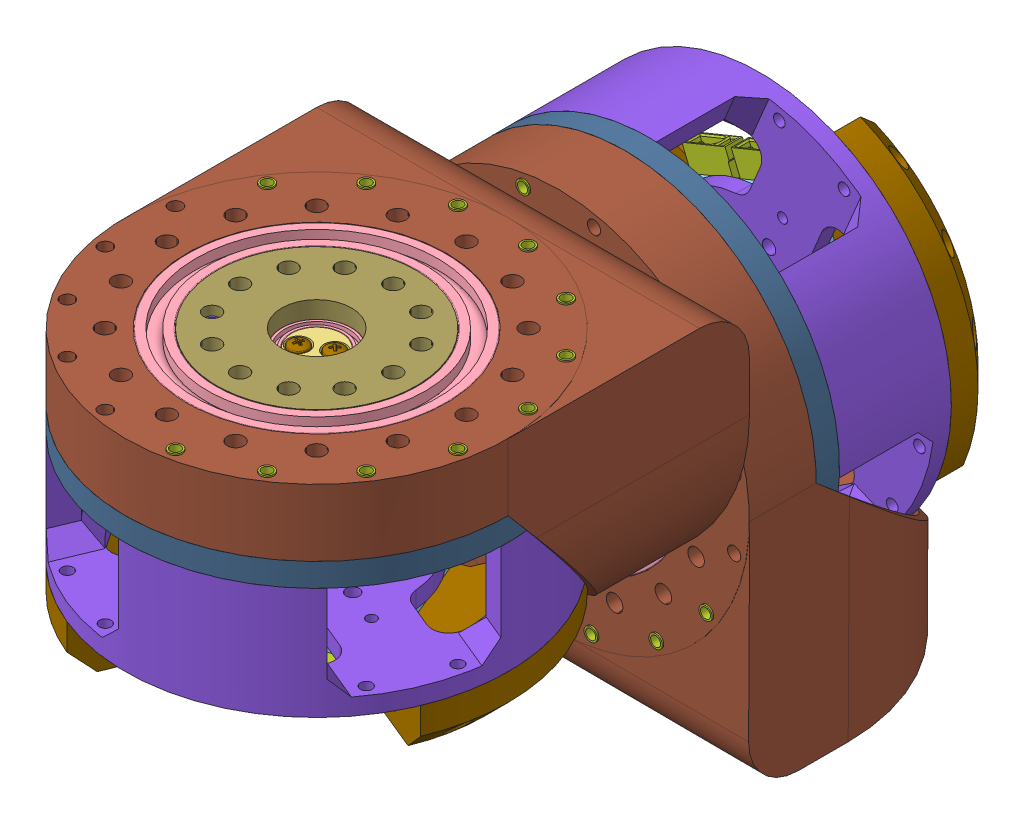
SolidWorks assembly hip, configuration Default. Lengths in mm.
Overall size (151.07 151.07 235.19).
696 component instances, 93 part files, 3 mates.
Components (placement in the parent):
- Cycloidal_v3-1: Cycloidal_v3 [Default] at (-2.6595 13.4678 32.6634) size (150.25 88 150.25)
  - motor-X83008S.stp-1: motor-X83008S.stp [Default] at (85.5027 89.8915 67.8666) x (-0.706334 0 0.707879) z (0 -1 0) size (114.7 114.7 37.62) (hidden)
    - base.stp-1: base.stp [Default] at (42.0794 12.0269 46.7342) size (91.6 91.6 15.61)
    - stator.stp-1: stator.stp [Default] at (42.0794 12.0269 33.1342) x (0.08493 -0.996387 0) z (0 0 1) size (83 83 8)
    - coil.stp-1: coil.stp [Default] at (39.5332 41.8984 37.1342) x (0.996387 0.08493 0) z (-0.08493 0.996387 0) size (4.4 10.2 10.5)
    - coil.stp-2: coil.stp [Default] at (34.3848 41.0025 37.1342) x (0.966502 0.256661 0) z (-0.256661 0.966502 0) size (4.4 10.2 10.5)
    - coil.stp-3: coil.stp [Default] at (29.4701 39.2261 37.1342) x (0.90725 0.420593 0) z (-0.420593 0.90725 0) size (4.4 10.2 10.5)
    - coil.stp-4: coil.stp [Default] at (24.9386 36.6233 37.1342) x (0.820431 0.571745 0) z (-0.571745 0.820431 0) size (4.4 10.2 10.5)
    - coil.stp-5: coil.stp [Default] at (20.9279 33.2732 37.1342) x (0.708685 0.705525 0) z (-0.705525 0.708685 0) size (4.4 10.2 10.5)
    - coil.stp-6: coil.stp [Default] at (17.5599 29.2775 37.1342) x (0.575405 0.817869 0) z (-0.817869 0.575405 0) size (4.4 10.2 10.5)
    - coil.stp-7: coil.stp [Default] at (14.9368 24.7576 37.1342) x (0.424642 0.905361 0) z (-0.905361 0.424642 0) size (4.4 10.2 10.5)
    - coil.stp-8: coil.stp [Default] at (13.1385 19.8509 37.1342) x (0.260976 0.965345 0) z (-0.965345 0.260976 0) size (4.4 10.2 10.5)
    - coil.stp-9: coil.stp [Default] at (12.2196 14.7066 37.1342) x (0.089381 0.995998 0) z (-0.995998 0.089381 0) size (4.4 10.2 10.5)
    - coil.stp-10: coil.stp [Default] at (12.2079 9.4807 37.1342) x (-0.08493 0.996387 0) z (-0.996387 -0.08493 0) size (4.4 10.2 10.5)
    - coil.stp-11: coil.stp [Default] at (13.1039 4.3323 37.1342) x (-0.256661 0.966502 0) z (-0.966502 -0.256661 0) size (4.4 10.2 10.5)
    - coil.stp-12: coil.stp [Default] at (14.8802 -0.5824 37.1342) x (-0.420593 0.90725 0) z (-0.90725 -0.420593 0) size (4.4 10.2 10.5)
    - coil.stp-13: coil.stp [Default] at (17.483 -5.1139 37.1342) x (-0.571745 0.820431 0) z (-0.820431 -0.571745 0) size (4.4 10.2 10.5)
    - coil.stp-14: coil.stp [Default] at (20.8332 -9.1246 37.1342) x (-0.705525 0.708685 0) z (-0.708685 -0.705525 0) size (4.4 10.2 10.5)
    - coil.stp-15: coil.stp [Default] at (24.8289 -12.4926 37.1342) x (-0.817869 0.575405 0) z (-0.575405 -0.817869 0) size (4.4 10.2 10.5)
    - coil.stp-16: coil.stp [Default] at (29.3487 -15.1157 37.1342) x (-0.905361 0.424642 0) z (-0.424642 -0.905361 0) size (4.4 10.2 10.5)
    - coil.stp-17: coil.stp [Default] at (34.2554 -16.914 37.1342) x (-0.965345 0.260976 0) z (-0.260976 -0.965345 0) size (4.4 10.2 10.5)
    - coil.stp-18: coil.stp [Default] at (39.3998 -17.8329 37.1342) x (-0.995998 0.089381 0) z (-0.089381 -0.995998 0) size (4.4 10.2 10.5)
    - coil.stp-19: coil.stp [Default] at (44.6256 -17.8446 37.1342) x (-0.996387 -0.08493 0) z (0.08493 -0.996387 0) size (4.4 10.2 10.5)
    - coil.stp-20: coil.stp [Default] at (49.7741 -16.9486 37.1342) x (-0.966502 -0.256661 0) z (0.256661 -0.966502 0) size (4.4 10.2 10.5)
    - coil.stp-21: coil.stp [Default] at (54.6887 -15.1723 37.1342) x (-0.90725 -0.420593 0) z (0.420593 -0.90725 0) size (4.4 10.2 10.5)
    - coil.stp-22: coil.stp [Default] at (59.2202 -12.5695 37.1342) x (-0.820431 -0.571745 0) z (0.571745 -0.820431 0) size (4.4 10.2 10.5)
    - coil.stp-23: coil.stp [Default] at (63.2309 -9.2193 37.1342) x (-0.708685 -0.705525 0) z (0.705525 -0.708685 0) size (4.4 10.2 10.5)
    - coil.stp-24: coil.stp [Default] at (66.599 -5.2236 37.1342) x (-0.575405 -0.817869 0) z (0.817869 -0.575405 0) size (4.4 10.2 10.5)
    - coil.stp-25: coil.stp [Default] at (69.222 -0.7038 37.1342) x (-0.424642 -0.905361 0) z (0.905361 -0.424642 0) size (4.4 10.2 10.5)
    - coil.stp-26: coil.stp [Default] at (71.0203 4.2029 37.1342) x (-0.260976 -0.965345 0) z (0.965345 -0.260976 0) size (4.4 10.2 10.5)
    - coil.stp-27: coil.stp [Default] at (71.9392 9.3473 37.1342) x (-0.089381 -0.995998 0) z (0.995998 -0.089381 0) size (4.4 10.2 10.5)
    - coil.stp-28: coil.stp [Default] at (71.9509 14.5731 37.1342) x (0.08493 -0.996387 0) z (0.996387 0.08493 0) size (4.4 10.2 10.5)
    - coil.stp-29: coil.stp [Default] at (71.055 19.7216 37.1342) x (0.256661 -0.966502 0) z (0.966502 0.256661 0) size (4.4 10.2 10.5)
    - coil.stp-30: coil.stp [Default] at (69.2786 24.6362 37.1342) x (0.420593 -0.90725 0) z (0.90725 0.420593 0) size (4.4 10.2 10.5)
    - coil.stp-31: coil.stp [Default] at (66.6758 29.1677 37.1342) x (0.571745 -0.820431 0) z (0.820431 0.571745 0) size (4.4 10.2 10.5)
    - coil.stp-32: coil.stp [Default] at (63.3257 33.1785 37.1342) x (0.705525 -0.708685 0) z (0.708685 0.705525 0) size (4.4 10.2 10.5)
    - coil.stp-33: coil.stp [Default] at (59.33 36.5465 37.1342) x (0.817869 -0.575405 0) z (0.575405 0.817869 0) size (4.4 10.2 10.5)
    - coil.stp-34: coil.stp [Default] at (54.8101 39.1695 37.1342) x (0.905361 -0.424642 0) z (0.424642 0.905361 0) size (4.4 10.2 10.5)
    - coil.stp-35: coil.stp [Default] at (49.9034 40.9678 37.1342) x (0.965345 -0.260976 0) z (0.260976 0.965345 0) size (4.4 10.2 10.5)
    - coil.stp-36: coil.stp [Default] at (44.759 41.8868 37.1342) x (0.995998 -0.089381 0) z (0.089381 0.995998 0) size (4.4 10.2 10.5)
    - rotor.stp-1: rotor.stp [Default] at (42.0794 12.0269 42.1342) x (-0.293442 0.955977 0) z (0 0 -1) size (91.8 91.8 12)
    - outrunner.stp-1: outrunner.stp [Default] at (42.0794 12.0269 30.1342) x (-0.254711 0.967017 0) z (-0.967017 -0.254711 0) size (91.8 17.01 91.8)
    - screw-mount.stp-1: screw-mount.stp [Default] at (38.1314 27.0157 27.1342) x (1 0 0) z (0 0 -1) size (7 7 6.5)
    - screw-mount.stp-2: screw-mount.stp [Default] at (27.0906 8.0789 27.1342) x (1 0 0) z (0 0 -1) size (7 7 6.5)
    - screw-mount.stp-3: screw-mount.stp [Default] at (57.0682 15.9749 27.1342) x (1 0 0) z (0 0 -1) size (7 7 6.5)
    - screw-mount.stp-4: screw-mount.stp [Default] at (46.0274 -2.9618 27.1342) x (1 0 0) z (0 0 -1) size (7 7 6.5)
    - 6702ZZ-bearing-15x21x4.stp-1: 6702ZZ-bearing-15x21x4.stp [Default] at (42.0794 12.0269 43.7342) x (1 0 0) z (0 -1 0) size (21 4 21)
    - 6702ZZ-bearing-15x21x4.stp-2: 6702ZZ-bearing-15x21x4.stp [Default] at (42.0794 12.0269 35.1342) x (1 0 0) z (0 1 0) size (21 4 21)
    - shaft.stp-1: shaft.stp [Default] at (42.0794 12.0269 20.1342) size (16 16 31.6)
    - fix-screw.stp-1: fix-screw.stp [Default] at (42.0794 12.0269 51.7342) x (1 0 0) z (0 0 -1) size (19.67 18.96 12.02)
  - Base_Plate-1: Base_Plate [Default] at (47.267 69.7573 89.1587) x (0.863342 0 -0.50462) z (0.50462 0 0.863342) size (40 7 40)
  - Eccentric_Shaft-1: Eccentric_Shaft [Default] at (38.9525 70.4165 102.8564) x (-0.50462 0 -0.863342) z (0.863342 0 -0.50462) size (20 15 17)
    - Eccentric_Shaft_bot-1: Eccentric_Shaft_bot [Default] at (7.6302 6.3409 14.0904) size (17 5 17)
    - Eccentric_Shaft_bot-2: Eccentric_Shaft_bot [Default] at (7.6302 11.3409 14.0904) x (-1 0 0) z (0 0 -1) size (17 5 17)
    - Eccentric_Shaft_top-1: Eccentric_Shaft_top [Default] at (7.6302 16.3409 14.0904) x (-1 0 0) z (0 0 -1) size (17 5 17)
  - radial ball bearing_68_iso-39: radial ball bearing_68_iso [ISO 15 RBB - 1860 - 32,SI,NC,32_68] at (47.267 91.8173 89.1587) x (0 1 0) z (0.105786 0 0.994389) size (10 78 78)
  - radial ball bearing_68_iso-40: radial ball bearing_68_iso [ISO 15 RBB - 1840 - 32,SI,NC,32_68] at (47.267 73.2573 89.1587) x (0 1 0) z (-0.019534 0 0.999809) size (7 52 52)
  - m13_bearing-31: m13_bearing [Default] at (-10.7414 95.4081 67.0593) x (0.227678 0 0.973736) z (0.973736 0 -0.227678) size (13 16 13)
    - m6-1: m6 [Default] at (8.4921 2.5508 14.8914) size (6 16 6)
    - radial ball bearing_68_iso-1: radial ball bearing_68_iso [ISO 15 RBB - 286 - 10,SI,NC,10_68] at (8.4921 16.0508 14.8914) x (0 1 0) z (0 0 1) size (5 13 13)
    - radial ball bearing_68_iso-2: radial ball bearing_68_iso [ISO 15 RBB - 286 - 10,SI,NC,10_68] at (8.4921 11.0508 14.8914) x (0 1 0) z (0 0 1) size (5 13 13)
  - m13_bearing-32: m13_bearing [Default] at (-14.1668 95.4081 84.2801) x (0.227678 0 0.973736) z (0.973736 0 -0.227678) size (13 16 13)
    - m6-1: m6 [Default] at (8.4921 2.5508 14.8914) size (6 16 6)
    - radial ball bearing_68_iso-1: radial ball bearing_68_iso [ISO 15 RBB - 286 - 10,SI,NC,10_68] at (8.4921 16.0508 14.8914) x (0 1 0) z (0 0 1) size (5 13 13)
    - radial ball bearing_68_iso-2: radial ball bearing_68_iso [ISO 15 RBB - 286 - 10,SI,NC,10_68] at (8.4921 11.0508 14.8914) x (0 1 0) z (0 0 1) size (5 13 13)
  - m13_bearing-34: m13_bearing [Default] at (13.6125 95.5581 125.8547) x (0.227678 0 0.973736) z (0.973736 0 -0.227678) size (13 16 13)
    - m6-1: m6 [Default] at (8.4921 2.5508 14.8914) size (6 16 6)
    - radial ball bearing_68_iso-1: radial ball bearing_68_iso [ISO 15 RBB - 286 - 10,SI,NC,10_68] at (8.4921 16.0508 14.8914) x (0 1 0) z (0 0 1) size (5 13 13)
    - radial ball bearing_68_iso-2: radial ball bearing_68_iso [ISO 15 RBB - 286 - 10,SI,NC,10_68] at (8.4921 11.0508 14.8914) x (0 1 0) z (0 0 1) size (5 13 13)
  - m13_bearing-35: m13_bearing [Default] at (-0.9866 95.4081 116.0999) x (0.227678 0 0.973736) z (0.973736 0 -0.227678) size (13 16 13)
    - m6-1: m6 [Default] at (8.4921 2.5508 14.8914) size (6 16 6)
    - radial ball bearing_68_iso-1: radial ball bearing_68_iso [ISO 15 RBB - 286 - 10,SI,NC,10_68] at (8.4921 16.0508 14.8914) x (0 1 0) z (0 0 1) size (5 13 13)
    - radial ball bearing_68_iso-2: radial ball bearing_68_iso [ISO 15 RBB - 286 - 10,SI,NC,10_68] at (8.4921 11.0508 14.8914) x (0 1 0) z (0 0 1) size (5 13 13)
  - m13_bearing-36: m13_bearing [Default] at (-10.7414 95.5581 101.5009) x (0.227678 0 0.973736) z (0.973736 0 -0.227678) size (13 16 13)
    - m6-1: m6 [Default] at (8.4921 2.5508 14.8914) size (6 16 6)
    - radial ball bearing_68_iso-1: radial ball bearing_68_iso [ISO 15 RBB - 286 - 10,SI,NC,10_68] at (8.4921 16.0508 14.8914) x (0 1 0) z (0 0 1) size (5 13 13)
    - radial ball bearing_68_iso-2: radial ball bearing_68_iso [ISO 15 RBB - 286 - 10,SI,NC,10_68] at (8.4921 11.0508 14.8914) x (0 1 0) z (0 0 1) size (5 13 13)
  - m13_bearing-1: m13_bearing [Default] at (-0.8801 95.4081 62.5627) x (0.736525 0 0.676411) z (0.676411 0 -0.736525) size (13 16 13)
    - m6-1: m6 [Default] at (8.4921 2.5508 14.8914) size (6 16 6)
    - radial ball bearing_68_iso-1: radial ball bearing_68_iso [ISO 15 RBB - 286 - 10,SI,NC,10_68] at (8.4921 16.0508 14.8914) x (0 1 0) z (0 0 1) size (5 13 13)
    - radial ball bearing_68_iso-2: radial ball bearing_68_iso [ISO 15 RBB - 286 - 10,SI,NC,10_68] at (8.4921 11.0508 14.8914) x (0 1 0) z (0 0 1) size (5 13 13)
  - m13_bearing-2: m13_bearing [Default] at (48.6831 95.4081 124.0939) x (0.120271 0 0.992741) z (0.992741 0 -0.120271) size (13 16 13)
    - m6-1: m6 [Default] at (8.4921 2.5508 14.8914) size (6 16 6)
    - radial ball bearing_68_iso-1: radial ball bearing_68_iso [ISO 15 RBB - 286 - 10,SI,NC,10_68] at (8.4921 16.0508 14.8914) x (0 1 0) z (0 0 1) size (5 13 13)
    - radial ball bearing_68_iso-2: radial ball bearing_68_iso [ISO 15 RBB - 286 - 10,SI,NC,10_68] at (8.4921 11.0508 14.8914) x (0 1 0) z (0 0 1) size (5 13 13)
  - m13_bearing-3: m13_bearing [Default] at (32.7832 95.4081 34.9886) x (-0.046141 0 0.998935) z (0.998935 0 0.046141) size (13 16 13)
    - m6-1: m6 [Default] at (8.4921 2.5508 14.8914) size (6 16 6)
    - radial ball bearing_68_iso-1: radial ball bearing_68_iso [ISO 15 RBB - 286 - 10,SI,NC,10_68] at (8.4921 16.0508 14.8914) x (0 1 0) z (0 0 1) size (5 13 13)
    - radial ball bearing_68_iso-2: radial ball bearing_68_iso [ISO 15 RBB - 286 - 10,SI,NC,10_68] at (8.4921 11.0508 14.8914) x (0 1 0) z (0 0 1) size (5 13 13)
  - m13_bearing-4: m13_bearing [Default] at (77.6928 95.3081 80.133) x (-0.036208 0 0.999344) z (0.999344 0 0.036208) size (13 16 13)
    - m6-1: m6 [Default] at (8.4921 2.5508 14.8914) size (6 16 6)
    - radial ball bearing_68_iso-1: radial ball bearing_68_iso [ISO 15 RBB - 286 - 10,SI,NC,10_68] at (8.4921 16.0508 14.8914) x (0 1 0) z (0 0 1) size (5 13 13)
    - radial ball bearing_68_iso-2: radial ball bearing_68_iso [ISO 15 RBB - 286 - 10,SI,NC,10_68] at (8.4921 11.0508 14.8914) x (0 1 0) z (0 0 1) size (5 13 13)
  - m13_bearing-5: m13_bearing [Default] at (73.474 95.4081 98.7828) x (0.059133 0 0.99825) z (0.99825 0 -0.059133) size (13 16 13)
    - m6-1: m6 [Default] at (8.4921 2.5508 14.8914) size (6 16 6)
    - radial ball bearing_68_iso-1: radial ball bearing_68_iso [ISO 15 RBB - 286 - 10,SI,NC,10_68] at (8.4921 16.0508 14.8914) x (0 1 0) z (0 0 1) size (5 13 13)
    - radial ball bearing_68_iso-2: radial ball bearing_68_iso [ISO 15 RBB - 286 - 10,SI,NC,10_68] at (8.4921 11.0508 14.8914) x (0 1 0) z (0 0 1) size (5 13 13)
  - m13_bearing-6: m13_bearing [Default] at (12.9248 95.4081 46.7315) x (0.451561 0 0.89224) z (0.89224 0 -0.451561) size (13 16 13)
    - m6-1: m6 [Default] at (8.4921 2.5508 14.8914) size (6 16 6)
    - radial ball bearing_68_iso-1: radial ball bearing_68_iso [ISO 15 RBB - 286 - 10,SI,NC,10_68] at (8.4921 16.0508 14.8914) x (0 1 0) z (0 0 1) size (5 13 13)
    - radial ball bearing_68_iso-2: radial ball bearing_68_iso [ISO 15 RBB - 286 - 10,SI,NC,10_68] at (8.4921 11.0508 14.8914) x (0 1 0) z (0 0 1) size (5 13 13)
  - m13_bearing-7: m13_bearing [Default] at (56.6452 95.4081 32.3406) x (-0.545813 0 0.837907) z (0.837907 0 0.545813) size (13 16 13)
    - m6-1: m6 [Default] at (8.4921 2.5508 14.8914) size (6 16 6)
    - radial ball bearing_68_iso-1: radial ball bearing_68_iso [ISO 15 RBB - 286 - 10,SI,NC,10_68] at (8.4921 16.0508 14.8914) x (0 1 0) z (0 0 1) size (5 13 13)
    - radial ball bearing_68_iso-2: radial ball bearing_68_iso [ISO 15 RBB - 286 - 10,SI,NC,10_68] at (8.4921 11.0508 14.8914) x (0 1 0) z (0 0 1) size (5 13 13)
  - m13_bearing-8: m13_bearing [Default] at (63.0373 95.4081 51.3153) x (0.158553 0 0.98735) z (0.98735 0 -0.158553) size (13 16 13)
    - m6-1: m6 [Default] at (8.4921 2.5508 14.8914) size (6 16 6)
    - radial ball bearing_68_iso-1: radial ball bearing_68_iso [ISO 15 RBB - 286 - 10,SI,NC,10_68] at (8.4921 16.0508 14.8914) x (0 1 0) z (0 0 1) size (5 13 13)
    - radial ball bearing_68_iso-2: radial ball bearing_68_iso [ISO 15 RBB - 286 - 10,SI,NC,10_68] at (8.4921 11.0508 14.8914) x (0 1 0) z (0 0 1) size (5 13 13)
  - m13_bearing-9: m13_bearing [Default] at (83.8577 95.4081 55.5358) x (-0.687134 0 0.72653) z (0.72653 0 0.687134) size (13 16 13)
    - m6-1: m6 [Default] at (8.4921 2.5508 14.8914) size (6 16 6)
    - radial ball bearing_68_iso-1: radial ball bearing_68_iso [ISO 15 RBB - 286 - 10,SI,NC,10_68] at (8.4921 16.0508 14.8914) x (0 1 0) z (0 0 1) size (5 13 13)
    - radial ball bearing_68_iso-2: radial ball bearing_68_iso [ISO 15 RBB - 286 - 10,SI,NC,10_68] at (8.4921 11.0508 14.8914) x (0 1 0) z (0 0 1) size (5 13 13)
  - m13_bearing-11: m13_bearing [Default] at (30.1977 95.4081 135.7424) x (0.57351 0 0.819198) z (0.819198 0 -0.57351) size (13 16 13)
    - m6-1: m6 [Default] at (8.4921 2.5508 14.8914) size (6 16 6)
    - radial ball bearing_68_iso-1: radial ball bearing_68_iso [ISO 15 RBB - 286 - 10,SI,NC,10_68] at (8.4921 16.0508 14.8914) x (0 1 0) z (0 0 1) size (5 13 13)
    - radial ball bearing_68_iso-2: radial ball bearing_68_iso [ISO 15 RBB - 286 - 10,SI,NC,10_68] at (8.4921 11.0508 14.8914) x (0 1 0) z (0 0 1) size (5 13 13)
  - m13_bearing-12: m13_bearing [Default] at (62.8861 95.4081 115.3744) x (0.184178 0 0.982893) z (0.982893 0 -0.184178) size (13 16 13)
    - m6-1: m6 [Default] at (8.4921 2.5508 14.8914) size (6 16 6)
    - radial ball bearing_68_iso-1: radial ball bearing_68_iso [ISO 15 RBB - 286 - 10,SI,NC,10_68] at (8.4921 16.0508 14.8914) x (0 1 0) z (0 0 1) size (5 13 13)
    - radial ball bearing_68_iso-2: radial ball bearing_68_iso [ISO 15 RBB - 286 - 10,SI,NC,10_68] at (8.4921 11.0508 14.8914) x (0 1 0) z (0 0 1) size (5 13 13)
  - socket button head screw_iso-2: socket button head screw_iso [ISO 7380 - M4 x 12 - 12N] at (47.267 67.4573 134.1587) x (0 1 0) z (-0.724148 0 0.689645) size (14.2 7.6 7.6)
  - socket button head screw_iso-3: socket button head screw_iso [ISO 7380 - M4 x 12 - 12N] at (15.4472 67.4573 57.3389) x (0 1 0) z (-0.724148 0 0.689645) size (14.2 7.6 7.6)
  - socket button head screw_iso-4: socket button head screw_iso [ISO 7380 - M4 x 12 - 12N] at (30.0462 67.4573 47.5841) x (0 1 0) z (-0.724148 0 0.689645) size (14.2 7.6 7.6)
  - socket button head screw_iso-5: socket button head screw_iso [ISO 7380 - M4 x 12 - 12N] at (47.267 67.4573 44.1587) x (0 1 0) z (-0.724148 0 0.689645) size (14.2 7.6 7.6)
  - socket button head screw_iso-6: socket button head screw_iso [ISO 7380 - M4 x 12 - 12N] at (64.4877 67.4573 47.5841) x (0 1 0) z (-0.724148 0 0.689645) size (14.2 7.6 7.6)
  - socket button head screw_iso-8: socket button head screw_iso [ISO 7380 - M4 x 12 - 12N] at (88.8416 67.4573 71.9379) x (0 1 0) z (-0.724148 0 0.689645) size (14.2 7.6 7.6)
  - socket button head screw_iso-9: socket button head screw_iso [ISO 7380 - M4 x 12 - 12N] at (92.267 67.4573 89.1587) x (0 1 0) z (-0.724148 0 0.689645) size (14.2 7.6 7.6)
  - socket button head screw_iso-10: socket button head screw_iso [ISO 7380 - M4 x 12 - 12N] at (88.8416 67.4573 106.3794) x (0 1 0) z (-0.724148 0 0.689645) size (14.2 7.6 7.6)
  - socket button head screw_iso-11: socket button head screw_iso [ISO 7380 - M4 x 12 - 12N] at (79.0868 67.4573 120.9785) x (0 1 0) z (-0.724148 0 0.689645) size (14.2 7.6 7.6)
  - M3x4x4.2_brass_insert-2: M3x4x4.2_brass_insert [Default] at (2.3676 97.2573 59.1579) x (-0.680278 0 -0.732954) z (-0.732954 0 0.680278) size (4 4 4)
  - M3x4x4.2_brass_insert-3: M3x4x4.2_brass_insert [Default] at (17.2662 97.2573 44.2593) x (-0.509546 0 -0.860444) z (-0.860444 0 0.509546) size (4 4 4)
  - M3x4x4.2_brass_insert-6: M3x4x4.2_brass_insert [Default] at (77.2678 97.2573 44.2593) x (-0.680278 0 -0.732954) z (-0.732954 0 0.680278) size (4 4 4)
  - M3x4x4.2_brass_insert-8: M3x4x4.2_brass_insert [Default] at (100.2294 93.2573 78.6238) x (-0.970393 0 0.241533) z (-0.241533 0 -0.970393) size (4 4 4)
  - M3x4x4.2_brass_insert-14: M3x4x4.2_brass_insert [Default] at (36.7321 97.2573 36.1963) x (0.509546 0 0.860444) z (0.860444 0 -0.509546) size (4 4 4)
  - M3x4x4.2_brass_insert-15: M3x4x4.2_brass_insert [Default] at (57.8019 93.2573 36.1963) x (0.897191 0 -0.441644) z (0.441644 0 0.897191) size (4 4 4)
  - M3x4x4.2_brass_insert-16: M3x4x4.2_brass_insert [Default] at (92.1663 97.2573 59.1579) x (-0.680278 0 -0.732954) z (-0.732954 0 0.680278) size (4 4 4)
  - M3x4x4.2_brass_insert-17: M3x4x4.2_brass_insert [Default] at (100.2294 97.2573 99.6935) x (0.680278 0 0.732954) z (0.732954 0 -0.680278) size (4 4 4)
  - M3x4x4.2_brass_insert-19: M3x4x4.2_brass_insert [Default] at (92.1663 97.2573 119.1595) x (0.680278 0 0.732954) z (0.732954 0 -0.680278) size (4 4 4)
  - M3x4x4.2_brass_insert-20: M3x4x4.2_brass_insert [Default] at (77.2678 97.2573 134.058) x (0.680278 0 0.732954) z (0.732954 0 -0.680278) size (4 4 4)
  - M3x4x4.2_brass_insert-21: M3x4x4.2_brass_insert [Default] at (57.8019 97.2573 142.1211) x (0.680278 0 0.732954) z (0.732954 0 -0.680278) size (4 4 4)
  - M4x6x5.5_brass_insert-47: M4x6x5.5_brass_insert [Default] at (5.6924 92.8573 71.9379) x (0.474598 0 0.880203) z (0 1 0) size (5 5 6)
  - M4x6x5.5_brass_insert-48: M4x6x5.5_brass_insert [Default] at (2.267 92.8573 89.1587) x (0.260051 0 0.965595) z (0 1 0) size (5 5 6)
  - M4x6x5.5_brass_insert-49: M4x6x5.5_brass_insert [Default] at (5.6924 87.0073 106.3794) x (-0.745833 0 0.666133) z (0 -1 0) size (5 5 6)
  - M4x6x5.5_brass_insert-50: M4x6x5.5_brass_insert [Default] at (15.4472 86.8573 120.9785) x (-0.745833 0 0.666133) z (0 -1 0) size (5 5 6)
  - M4x6x5.5_brass_insert-51: M4x6x5.5_brass_insert [Default] at (30.0462 87.0073 130.7332) x (0.260051 0 -0.965595) z (0 -1 0) size (5 5 6)
  - M4x6x5.5_brass_insert-6: M4x6x5.5_brass_insert [Default] at (27.3484 93.9895 100.6587) x (0.252509 0 0.967595) z (0 1 0) size (5 5 6)
  - M4x6x5.5_brass_insert-20: M4x6x5.5_brass_insert [Default] at (64.4877 86.8573 130.7332) x (-0.745833 0 0.666133) z (0 -1 0) size (5 5 6)
  - M4x6x5.5_brass_insert-21: M4x6x5.5_brass_insert [Default] at (47.267 86.8573 134.1587) x (-0.745833 0 0.666133) z (0 -1 0) size (5 5 6)
  - M4x6x5.5_brass_insert-22: M4x6x5.5_brass_insert [Default] at (15.4472 86.8573 57.3389) x (0.623293 0 0.781988) z (0 -1 0) size (5 5 6)
  - M4x6x5.5_brass_insert-23: M4x6x5.5_brass_insert [Default] at (30.0462 86.8573 47.5841) x (0.623293 0 0.781988) z (0 -1 0) size (5 5 6)
  - M4x6x5.5_brass_insert-24: M4x6x5.5_brass_insert [Default] at (79.0868 86.8573 120.9785) x (0.541965 0 0.840401) z (0 -1 0) size (5 5 6)
  - M4x6x5.5_brass_insert-25: M4x6x5.5_brass_insert [Default] at (88.8416 86.8573 106.3794) x (-0.745833 0 0.666133) z (0 -1 0) size (5 5 6)
  - M4x6x5.5_brass_insert-26: M4x6x5.5_brass_insert [Default] at (92.267 86.8573 89.1587) x (-0.745833 0 0.666133) z (0 -1 0) size (5 5 6)
  - M4x6x5.5_brass_insert-27: M4x6x5.5_brass_insert [Default] at (88.8416 86.8573 71.9379) x (-0.745833 0 0.666133) z (0 -1 0) size (5 5 6)
  - M4x6x5.5_brass_insert-28: M4x6x5.5_brass_insert [Default] at (79.0868 92.8573 57.3389) x (0.260051 0 0.965595) z (0 1 0) size (5 5 6)
  - M4x6x5.5_brass_insert-29: M4x6x5.5_brass_insert [Default] at (64.4877 86.8573 47.5841) x (-0.142939 0 0.989731) z (0 -1 0) size (5 5 6)
  - M4x6x5.5_brass_insert-31: M4x6x5.5_brass_insert [Default] at (47.267 86.8573 44.1587) x (-0.220341 0 0.975423) z (0 -1 0) size (5 5 6)
  - pan cross head_am-1: pan cross head_am [B18.6.7M - M3 x 0.5 x 20 Type I Cross Recessed PHMS --20N] at (50.7204 92.6573 87.1402) x (0 -1 0) z (0.748822 0 0.662771) size (22.37 5.6 5.6)
  - pan cross head_am-3: pan cross head_am [B18.6.7M - M3 x 0.5 x 20 Type I Cross Recessed PHMS --20N] at (43.8136 92.6573 91.1771) x (0 -1 0) z (0.940321 0 0.340288) size (22.37 5.6 5.6)
  - M3x4x4.2_brass_insert-22: M3x4x4.2_brass_insert [Default] at (50.7204 69.7573 87.1402) x (0.984485 0 -0.175469) z (0.175469 0 0.984485) size (4 4 4)
  - M3x4x4.2_brass_insert-23: M3x4x4.2_brass_insert [Default] at (43.8136 69.7573 91.1771) x (0.984609 0 -0.174769) z (0.174769 0 0.984609) size (4 4 4)
  - pan cross head_am-4: pan cross head_am [B18.6.7M - M3 x 0.5 x 10 Type I Cross Recessed PHMS --10N] at (33.8852 77.6573 96.9803) x (0 -1 0) z (0 0 1) size (12.37 5.6 5.6)
  - pan cross head_am-5: pan cross head_am [B18.6.7M - M3 x 0.5 x 10 Type I Cross Recessed PHMS --10N] at (60.6488 77.6573 81.3371) x (0 -1 0) z (0 0 1) size (12.37 5.6 5.6)
  - pan cross head_am-6: pan cross head_am [B18.6.7M - M3 x 0.5 x 10 Type I Cross Recessed PHMS --10N] at (55.0886 77.6573 102.5405) x (0 -1 0) z (0 0 1) size (12.37 5.6 5.6)
  - pan cross head_am-7: pan cross head_am [B18.6.7M - M3 x 0.5 x 10 Type I Cross Recessed PHMS --10N] at (39.4454 77.6573 75.7769) x (0 -1 0) z (0 0 1) size (12.37 5.6 5.6)
  - radial ball bearing_68_iso-44: radial ball bearing_68_iso [ISO 15 RBB - 1715 - 26,SI,NC,26_68] at (46.5101 84.7573 87.8637) x (0 1 0) z (-0.714953 0 -0.699173) size (4 21 21)
  - radial ball bearing_68_iso-45: radial ball bearing_68_iso [ISO 15 RBB - 1715 - 26,SI,NC,26_68] at (47.267 89.7573 89.1587) x (0 1 0) z (0.999483 0 -0.032163) size (4 21 21)
  - radial ball bearing_68_iso-46: radial ball bearing_68_iso [ISO 15 RBB - 1715 - 26,SI,NC,26_68] at (48.0239 79.7573 90.4537) x (0 1 0) z (0.000644 0 1) size (4 21 21)
  - socket button head screw_iso-37: socket button head screw_iso [ISO 7380 - M4 x 12 - 12N] at (79.0868 67.4573 57.3389) x (0 1 0) z (-0.709975 0 0.704227) size (14.2 7.6 7.6)
  - socket button head screw_iso-38: socket button head screw_iso [ISO 7380 - M4 x 12 - 12N] at (64.4877 67.4573 130.7332) x (0 1 0) z (-0.724148 0 0.689645) size (14.2 7.6 7.6)
  - foc-motor-controller.step-1: foc-motor-controller.step [Default] at (47.267 33.7573 89.1587) x (-0.382683 0 -0.92388) z (0 -1 0) size (57.23 50 8.13)
    - RTA0040B.step-1: RTA0040B.step [Default] at (12.5014 -1.6986 1.595) x (-0.707107 -0.707107 0) z (0 0 1) size (6 6 1)
      - FRAME.step-1: FRAME.step [Default] x (1 0 0) z (0 -1 0) size (6 0.2 6)
        - SOLID.step-1: SOLID.step [Default] at origin size (0.4 0.2 0.22)
        - SOLID-0.step-1: SOLID-0.step [Default] at origin size (0.4 0.2 0.22)
        - SOLID-1.step-1: SOLID-1.step [Default] at origin size (0.4 0.2 0.22)
        - SOLID-2.step-1: SOLID-2.step [Default] at origin size (0.4 0.2 0.22)
        - SOLID-3.step-1: SOLID-3.step [Default] at origin size (0.4 0.2 0.22)
        - SOLID-4.step-1: SOLID-4.step [Default] at origin size (0.4 0.2 0.22)
        - SOLID-5.step-1: SOLID-5.step [Default] at origin size (0.4 0.2 0.22)
        - SOLID-6.step-1: SOLID-6.step [Default] at origin size (0.4 0.2 0.22)
        - SOLID-7.step-1: SOLID-7.step [Default] at origin size (0.4 0.2 0.22)
        - SOLID-8.step-1: SOLID-8.step [Default] at origin size (0.4 0.2 0.22)
        - SOLID-9.step-1: SOLID-9.step [Default] at origin size (0.22 0.2 0.4)
        - SOLID-10.step-1: SOLID-10.step [Default] at origin size (0.22 0.2 0.4)
        - SOLID-11.step-1: SOLID-11.step [Default] at origin size (0.22 0.2 0.4)
        - SOLID-12.step-1: SOLID-12.step [Default] at origin size (0.22 0.2 0.4)
        - SOLID-13.step-1: SOLID-13.step [Default] at origin size (0.22 0.2 0.4)
        - SOLID-14.step-1: SOLID-14.step [Default] at origin size (0.22 0.2 0.4)
        - SOLID-15.step-1: SOLID-15.step [Default] at origin size (0.22 0.2 0.4)
        - SOLID-16.step-1: SOLID-16.step [Default] at origin size (0.22 0.2 0.4)
        - SOLID-17.step-1: SOLID-17.step [Default] at origin size (4.15 0.2 4.15)
        - SOLID-18.step-1: SOLID-18.step [Default] at origin size (0.28 0.1 0.28)
        - SOLID-19.step-1: SOLID-19.step [Default] at origin size (0.28 0.1 0.28)
        - SOLID-20.step-1: SOLID-20.step [Default] at origin size (0.28 0.1 0.28)
        - SOLID-21.step-1: SOLID-21.step [Default] at origin size (0.28 0.1 0.28)
        - SOLID-22.step-1: SOLID-22.step [Default] at origin size (0.4 0.2 0.22)
        - SOLID-23.step-1: SOLID-23.step [Default] at origin size (0.4 0.2 0.22)
        - SOLID-24.step-1: SOLID-24.step [Default] at origin size (0.4 0.2 0.22)
        - SOLID-25.step-1: SOLID-25.step [Default] at origin size (0.4 0.2 0.22)
        - SOLID-26.step-1: SOLID-26.step [Default] at origin size (0.4 0.2 0.22)
        - SOLID-27.step-1: SOLID-27.step [Default] at origin size (0.4 0.2 0.22)
        - SOLID-28.step-1: SOLID-28.step [Default] at origin size (0.4 0.2 0.22)
        - SOLID-29.step-1: SOLID-29.step [Default] at origin size (0.4 0.2 0.22)
        - SOLID-30.step-1: SOLID-30.step [Default] at origin size (0.4 0.2 0.22)
        - SOLID-31.step-1: SOLID-31.step [Default] at origin size (0.4 0.2 0.22)
        - SOLID-32.step-1: SOLID-32.step [Default] at origin size (0.22 0.2 0.4)
        - SOLID-33.step-1: SOLID-33.step [Default] at origin size (0.22 0.2 0.4)
        - SOLID-34.step-1: SOLID-34.step [Default] at origin size (0.22 0.2 0.4)
        - SOLID-35.step-1: SOLID-35.step [Default] at origin size (0.22 0.2 0.4)
        - SOLID-36.step-1: SOLID-36.step [Default] at origin size (0.22 0.2 0.4)
        - SOLID-37.step-1: SOLID-37.step [Default] at origin size (0.22 0.2 0.4)
        - SOLID-38.step-1: SOLID-38.step [Default] at origin size (0.22 0.2 0.4)
        - SOLID-39.step-1: SOLID-39.step [Default] at origin size (0.22 0.2 0.4)
        - SOLID-40.step-1: SOLID-40.step [Default] at origin size (0.22 0.2 0.4)
        - SOLID-41.step-1: SOLID-41.step [Default] at origin size (0.22 0.2 0.4)
        - SOLID-42.step-1: SOLID-42.step [Default] at origin size (0.22 0.2 0.4)
        - SOLID-43.step-1: SOLID-43.step [Default] at origin size (0.22 0.2 0.4)
      - BODY.step-1: BODY.step [Default] at (0 0 0.025) x (1 0 0) z (0 -1 0) size (6 0.97 6)
    - Resonator_SMD_Murata_CSTxExxV-3Pin_3.0x1.1mm.step-1: Resonator_SMD_Murata_CSTxExxV-3Pin_3.0x1.1mm.step [Default] at (1.8 -7 1.595) x (0 1 0) z (0 0 1) size (3.2 1.35 0.9)
    - C_0603_1608Metric.step-1: C_0603_1608Metric.step [Default] at (6.2 -16.8 1.595) x (0 -1 0) z (0 0 1) size (1.6 0.8 0.8)
    - R_0603_1608Metric.step-1: R_0603_1608Metric.step [Default] at (11.8 -7.375 1.595) x (0 1 0) z (0 0 1) size (1.6 0.8 0.45)
    - R_0603_1608Metric.step-2: R_0603_1608Metric.step [Default] at (13.8 -16.8 1.595) x (0 1 0) z (0 0 1) size (1.6 0.8 0.45)
    - R_0603_1608Metric.step-3: R_0603_1608Metric.step [Default] at (18.1 -5.36 1.595) size (1.6 0.8 0.45)
    - C_0603_1608Metric.step-2: C_0603_1608Metric.step [Default] at (2.6 -0.5 1.595) x (0 -1 0) z (0 0 1) size (1.6 0.8 0.8)
    - R_0603_1608Metric.step-4: R_0603_1608Metric.step [Default] at (14.6 -11.3 1.595) x (0 1 0) z (0 0 1) size (1.6 0.8 0.45)
    - L_APV_ANR4020.step-1: L_APV_ANR4020.step [Default] at (22.3 -13.7 1.595) x (0 -1 0) z (0 0 1) size (4.02 4 2)
    - C_0603_1608Metric.step-3: C_0603_1608Metric.step [Default] at (0.3 -12.6 1.595) x (-1 0 0) z (0 0 1) size (1.6 0.8 0.8)
    - C_1206_3216Metric.step-1: C_1206_3216Metric.step [Default] at (15.7 11 1.595) x (0 1 0) z (0 0 1) size (3.2 1.6 1.6)
    - C_0603_1608Metric.step-4: C_0603_1608Metric.step [Default] at (0.3 -9.6 1.595) size (1.6 0.8 0.8)
    - R_0603_1608Metric.step-5: R_0603_1608Metric.step [Default] at (12.3 -16.8 1.595) x (0 1 0) z (0 0 1) size (1.6 0.8 0.45)
    - C_0603_1608Metric.step-5: C_0603_1608Metric.step [Default] at (-0.3 -16.6 1.595) x (0 1 0) z (0 0 1) size (1.6 0.8 0.8)
    - R_0603_1608Metric.step-6: R_0603_1608Metric.step [Default] at (10.9 4.1 1.595) size (1.6 0.8 0.45)
    - C_1206_3216Metric.step-2: C_1206_3216Metric.step [Default] at (6.3 11 1.595) x (0 1 0) z (0 0 1) size (3.2 1.6 1.6)
    - XT30PW_2_2_-M.G.B.step-1: XT30PW_2_2_-M.G.B.step [Default] at (-20.5 9.5 1.595) x (0 -1 0) z (-1 0 0) size (15.5 7.1 12.53)
    - R_0603_1608Metric.step-7: R_0603_1608Metric.step [Default] at (0.3 -11.1 1.595) size (1.6 0.8 0.45)
    - C_0603_1608Metric.step-6: C_0603_1608Metric.step [Default] at (19 -0.4 1.595) x (-0.707107 -0.707107 0) z (0 0 1) size (1.6 0.8 0.8)
    - C_1206_3216Metric.step-3: C_1206_3216Metric.step [Default] at (13.3 11 1.595) x (0 1 0) z (0 0 1) size (3.2 1.6 1.6)
    - R_0603_1608Metric.step-8: R_0603_1608Metric.step [Default] at (10.2 -7.375 1.595) x (0 -1 0) z (0 0 1) size (1.6 0.8 0.45)
    - JST_GH_SM08B-GHS-TB_1x08-1MP_P1.25mm_Horizontal.step-1: JST_GH_SM08B-GHS-TB_1x08-1MP_P1.25mm_Horizontal.step [Default] at (10 -22 1.595) size (13.25 4.95 4.25)
    - C_1206_3216Metric.step-4: C_1206_3216Metric.step [Default] at (-12.3 11 1.595) x (0 1 0) z (0 0 1) size (3.2 1.6 1.6)
    - JST_GH_SM06B-GHS-TB_1x06-1MP_P1.25mm_Horizontal.step-1: JST_GH_SM06B-GHS-TB_1x06-1MP_P1.25mm_Horizontal.step [Default] at (-4.3 -22 1.595) size (10.75 4.95 4.25)
    - C_0603_1608Metric.step-7: C_0603_1608Metric.step [Default] at (7.3 -4.5 1.595) x (-1 0 0) z (0 0 1) size (1.6 0.8 0.8)
    - R_0603_1608Metric.step-9: R_0603_1608Metric.step [Default] at (18.1 -3.86 1.595) x (-1 0 0) z (0 0 1) size (1.6 0.8 0.45)
    - C_1206_3216Metric.step-5: C_1206_3216Metric.step [Default] at (22.6794 -1.2206 1.595) x (0.707107 -0.707107 0) z (0 0 1) size (3.2 1.6 1.6)
    - R_Array_Convex_4x0402.step-1: R_Array_Convex_4x0402.step [Default] at (6.8 -2.5 1.595) size (1 2 0.35)
    - R_0603_1608Metric.step-10: R_0603_1608Metric.step [Default] at (7.7 -16.8 1.595) x (0 -1 0) z (0 0 1) size (1.6 0.8 0.45)
    - C_1206_3216Metric.step-6: C_1206_3216Metric.step [Default] at (8.7 11 1.595) x (0 1 0) z (0 0 1) size (3.2 1.6 1.6)
    - C_0603_1608Metric.step-8: C_0603_1608Metric.step [Default] at (16.1 -11.3 1.595) x (0 1 0) z (0 0 1) size (1.6 0.8 0.8)
    - SOT-23-5.step-1: SOT-23-5.step [Default] at (-3.1 -16.6 1.595) x (-1 0 0) z (0 0 1) size (2.8 2.9 1.55)
    - C_0603_1608Metric.step-9: C_0603_1608Metric.step [Default] at (17.8 -13.6 1.595) size (1.6 0.8 0.8)
    - R_0603_1608Metric.step-11: R_0603_1608Metric.step [Default] at (-11.5 -20.3875 1.595) x (0 -1 0) z (0 0 1) size (1.6 0.8 0.45)
    - C_0603_1608Metric.step-10: C_0603_1608Metric.step [Default] at (-12.4 2.3 1.595) x (0 1 0) z (0 0 1) size (1.6 0.8 0.8)
    - C_1206_3216Metric.step-7: C_1206_3216Metric.step [Default] at (18 11 1.595) x (0 1 0) z (0 0 1) size (3.2 1.6 1.6)
    - R_0603_1608Metric.step-12: R_0603_1608Metric.step [Default] at (-10.8105 -14.9971 1.595) x (-1 0 0) z (0 0 1) size (1.6 0.8 0.45)
    - C_0603_1608Metric.step-11: C_0603_1608Metric.step [Default] at (-13.8 -9.4 1.595) x (-1 0 0) z (0 0 1) size (1.6 0.8 0.8)
    - R_0603_1608Metric.step-13: R_0603_1608Metric.step [Default] at (-23.15 -14.5 1.595) x (-1 0 0) z (0 0 1) size (1.6 0.8 0.45)
    - C_0603_1608Metric.step-12: C_0603_1608Metric.step [Default] at (1.1 -0.2 1.595) x (0 1 0) z (0 0 1) size (1.6 0.8 0.8)
    - D_0805_2012Metric.step-1: D_0805_2012Metric.step [Default] at (22.9 -9.6 1.595) x (0 1 0) z (0 0 1) size (2 1.27 0.8)
    - C_0603_1608Metric.step-13: C_0603_1608Metric.step [Default] at (-7.8 3.775 1.595) x (0 -1 0) z (0 0 1) size (1.6 0.8 0.8)
    - R_0603_1608Metric.step-14: R_0603_1608Metric.step [Default] at (-6.4 -12.825 1.595) x (0 1 0) z (0 0 1) size (1.6 0.8 0.45)
    - L_0603_1608Metric.step-1: L_0603_1608Metric.step [Default] at (-10.1 3 1.595) size (1.6 0.8 0.8)
    - C_0603_1608Metric.step-14: C_0603_1608Metric.step [Default] at (17.9 0.7 1.595) x (-0.707107 -0.707107 0) z (0 0 1) size (1.6 0.8 0.8)
    - HVSSOP-10.step-1: HVSSOP-10.step [Default] at (18.6 -9.6 1.595) x (0 -1 0) z (-1 0 0) size (4.9 1.1 3)
    - C_0603_1608Metric.step-15: C_0603_1608Metric.step [Default] at (7.9 4.1 1.595) x (-1 0 0) z (0 0 1) size (1.6 0.8 0.8)
    - C_0603_1608Metric.step-16: C_0603_1608Metric.step [Default] at (21.1 -9.6 1.595) x (0 -1 0) z (0 0 1) size (1.6 0.8 0.8)
    - R_0603_1608Metric.step-15: R_0603_1608Metric.step [Default] at (-10.8105 -11.9971 1.595) x (-1 0 0) z (0 0 1) size (1.6 0.8 0.45)
    - R_0603_1608Metric.step-16: R_0603_1608Metric.step [Default] at (-18.2 -17.4 1.595) size (1.6 0.8 0.45)
    - C_1206_3216Metric.step-8: C_1206_3216Metric.step [Default] at (-3 11 1.595) x (0 1 0) z (0 0 1) size (3.2 1.6 1.6)
    - R_0603_1608Metric.step-17: R_0603_1608Metric.step [Default] at (-16.9 -20.4 1.595) x (0 -1 0) z (0 0 1) size (1.6 0.8 0.45)
